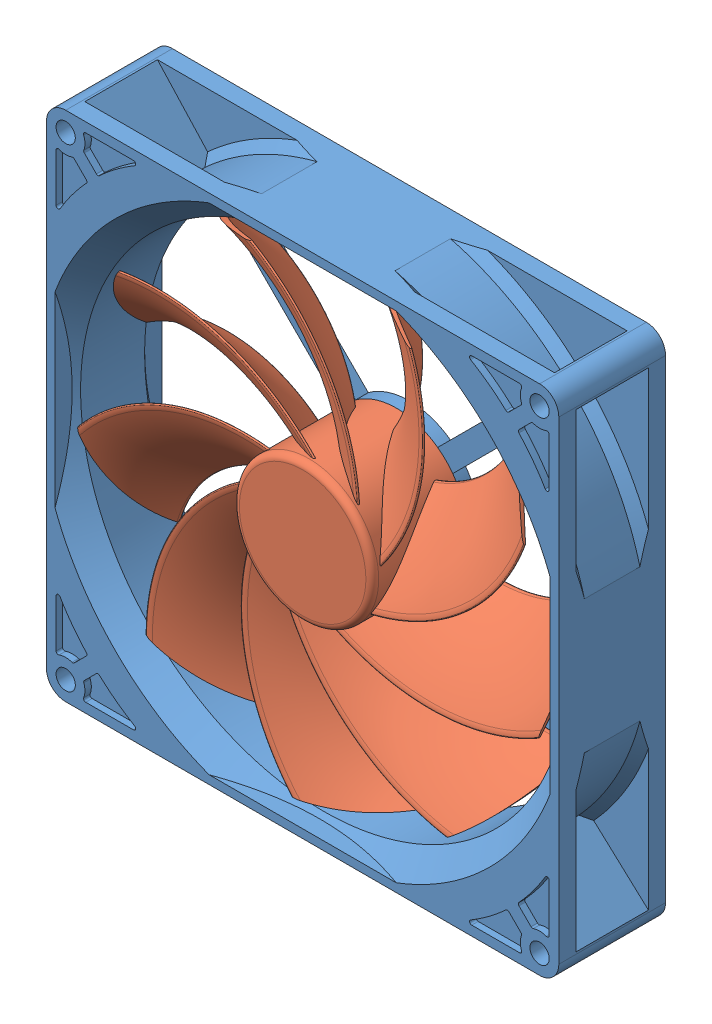
SolidWorks assembly PC FAN, configuration Default. Lengths in mm.
Overall size (183.81 183.8 33.39).
2 component instances, 2 part files, 2 mates.
Components (placement in the parent):
- CPU Fan 1-1: CPU Fan 1 [Default] at origin size (120 120 33.39)
- Part3^PC FAN-1: Part3^PC FAN [Default] at (0 0 -9.5) x (-0.828072 -0.560621 0) z (0 0 1) size (132.38 132.34 22) (virtual)
Mates (geometry in assembly coordinates):
- Coincident5: coincident: plane of CPU Fan 1-1 through (0 0 -9.5) normal (0 0 1); plane of Part3^PC FAN-1 through (0 0 -9.5) normal (0 0 -1)
- Concentric1: concentric: cylinder of CPU Fan 1-1 through (0 0 -9.5) axis (0 0 -1) radius 16.3; cylinder of Part3^PC FAN-1 through (0 0 12.5) axis (0 0 -1) radius 16.3
